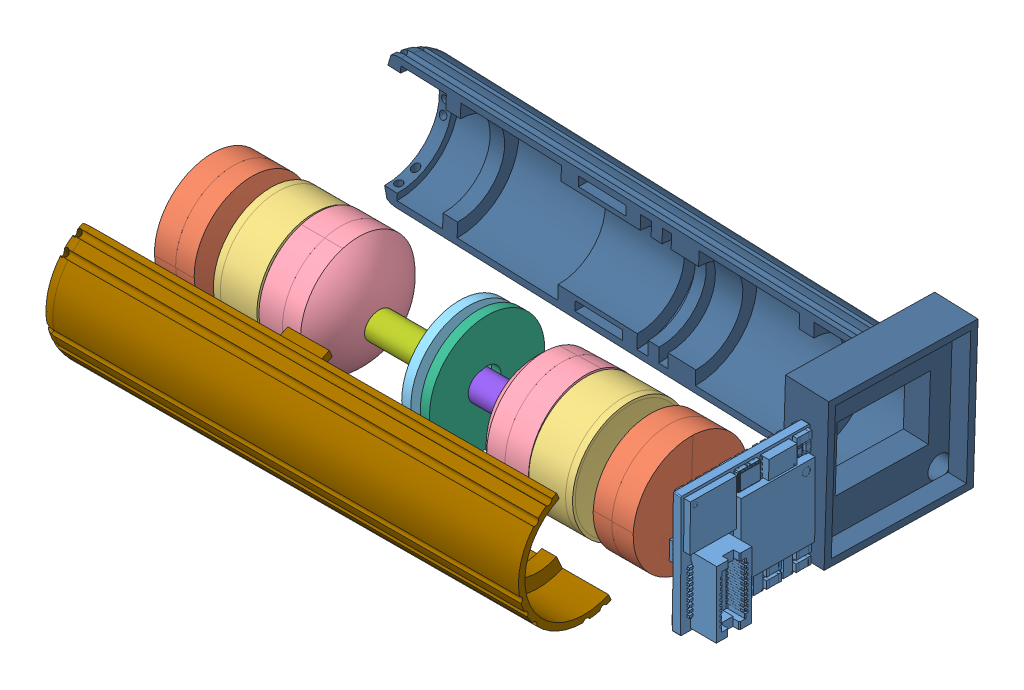
SolidWorks assembly Assem_disassembled_light_holders_20250226, configuration Default. Lengths in mm.
Overall size (63.85 18.24 48.22).
14 component instances, 11 part files, 0 mates.
Components (placement in the parent):
- MU9-MH-BRD.stp-1: MU9-MH-BRD.stp [Default] at (54.1184 7.8553 -8.606) x (-0.005156 0.003988 0.999979) z (0.999983 -0.002731 0.005166) size (13.9 13.11 5.52)
- step_49660.step-1: step_49660.step [Default] at (1.8179 8.0621 -8.6172) x (-0.003014 -0.039967 0.999196) z (-0.999995 0.001187 -0.002969) size (12.5 12.5 5.58)
- step_45424.stp-1: step_45424.stp [Default] at (6.5717 8.0488 -8.6275) x (-0.001186 0.992643 -0.12107) z (-0.99999 -0.001688 -0.004044) size (12.5 12.5 4.74)
- step_49658.step-1: step_49658.step [Default] at (14.8917 8.0055 -8.7316) x (-0.013096 -0.962776 -0.269982) z (-0.999895 0.010947 0.009462) size (12.5 12.5 8.08)
- step_45424.stp-2: step_45424.stp [Default] at (37.8896 7.5265 -8.426) x (0.006091 -0.99469 -0.102732) z (0.999979 0.006262 -0.001345) size (12.5 12.5 4.74)
- step_49660.step-2: step_49660.step [Default] at (42.8807 7.6649 -8.3606) x (0.003014 0.039967 0.999196) z (0.999995 -0.001187 -0.002969) size (12.5 12.5 5.58)
- step_49658.step-2: step_49658.step [Default] at (29.5702 7.5016 -8.2686) x (-0.017181 0.953966 -0.299421) z (0.999748 0.01207 -0.01891) size (12.5 12.5 8.08)
- filter-1: filter [Default] at (23.1251 7.6742 -8.5853) x (0 1 0) z (0 0 -1) size (12.5 1 12.5)
- Mask-1: Mask [Default] at (25.0866 7.7311 -8.6397) x (0 0 -1) z (0 -1 0) size (12.5 1 12.5)
- lightCone1-1: lightCone1 [Default] at (-6.8234 7.5792 -8.278) size (30 3 3)
- lightCone2-1: lightCone2 [Default] at (24.0672 7.6044 -8.0853) size (27.94 3 3)
- Part1^Assem_disassembled_light_holders_20250226-1: Part1^Assem_disassembled_light_holders_20250226 [Default] at origin (virtual)
- optics_holder_nocap-p2-0820-1: optics_holder_nocap-p2-0820 [Default] at (14.941 15.5651 6.0362) x (0.999993 0.003733 -0.000354) z (-0.00187 0.414458 -0.910067) size (51.82 14.26 8.4)
- optics_holder_withcam3.0-p1-0820-1: optics_holder_withcam3.0-p1-0820 [Default] at (14.5775 -0.1004 -27.2717) x (0.999623 -0.024557 0.012257) z (-0.012079 0.007369 0.9999) size (56.57 16 16)
